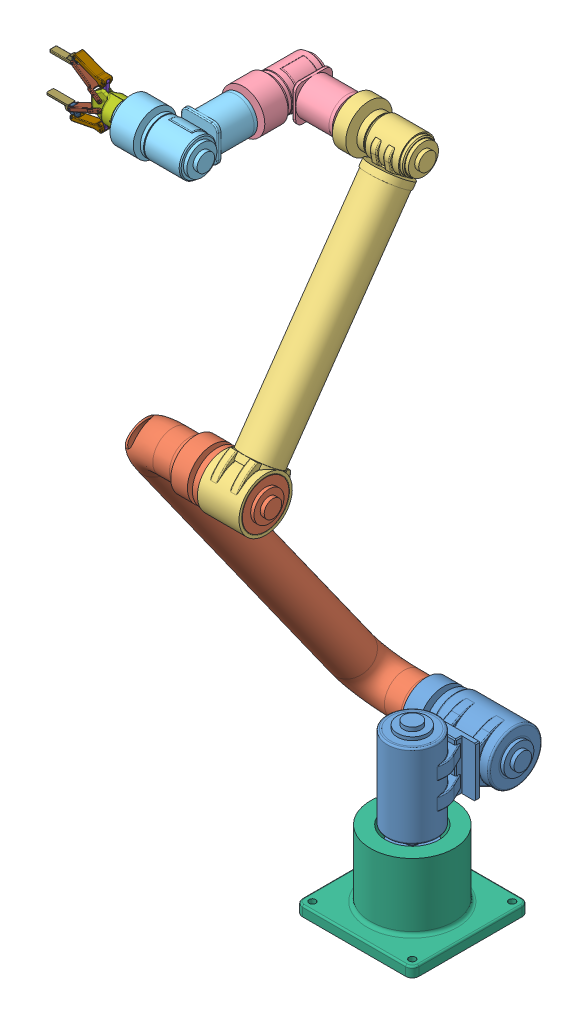
SolidWorks assembly qf_space_manipilator, configuration 默认. Lengths in mm.
Overall size (931.68 2266.25 1901.05).
18 component instances, 12 part files, 19 mates.
Components (placement in the parent):
- 1-1: 1 [默认] at (175 480 1283.54) x (1 0 0) z (0 -1 0) size (296.02 355 322)
- 2-1: 2 [默认] at (10.98 360 1083.54) x (0 -0.094498 0.995525) z (1 0 0) size (741.96 1181.19 535.98)
- 3-1: 3 [默认] at (167.5 1403.4778 1733.2672) x (0 0.572418 0.819962) z (0 0.819962 -0.572418) size (161.46 230.6 965)
- 4-1: 4 [默认] at (8.9 2006.1499 1312.54) x (0 1 0) z (1 0 0) size (130 235 470.6)
- 5-1: 5 [默认] at (763.6983 2411.2318 -1009.3375) x (-0.587026 0.762889 0.270927) z (-0.805463 -0.584033 -0.100675) size (262.23 449.62 237.88)
- Main_carrier_of_spool_cover_Varsay_X2_0131_X0_lan-1: Main_carrier_of_spool_cover_Varsay_X2_0131_X0_lan [默认] at (175 0 1283.54) x (0 0 1) z (0 1 0) size (350 350 230)
- Robotiq 2f-140-1: Robotiq 2f-140 [默认] at (-742.3808 2088.878 1773.5387) x (0.739353 0.591715 0.321296) z (0.557602 -0.805552 0.200415) size (250.11 134.48 238.85)
  - 2F-Body-1: 2F-Body [默认] at (218.7669 -271.2651 273.3125) x (0.593526 -0.031903 -0.804182) z (0.321296 0.925528 0.200415) size (89.6 94.04 75)
  - Finger1-1: Finger1 [默认] at (213.3406 -273.1738 290.8261) x (0.782068 -0.139996 -0.607265) z (0.321296 0.925528 0.200415) size (33.04 20.16 9.4)
  - Finger1-2: Finger1 [默认] at (225.7111 -272.8186 269.3539) x (-0.493154 -0.017144 0.869773) z (-0.321296 -0.925528 -0.200415) size (33.04 20.16 9.4)
  - Finger2-1: Finger2 [默认] at (213.3406 -273.1738 290.8261) x (0.782068 -0.139996 -0.607265) z (0.321296 0.925528 0.200415) size (58 91.26 27.21)
  - Finger4-1: Finger4 [默认] at (221.3264 -265.9336 244.5877) x (0.593526 -0.031903 -0.804182) z (0.321296 0.925528 0.200415) size (29.9 28.02 27)
  - Finger3-1: Finger3 [默认] at (208.6208 -271.1191 288.6542) x (0.782068 -0.139996 -0.607265) z (0.321296 0.925528 0.200415) size (78.86 86.37 35.78)
  - Fingertip-1: Fingertip [默认] at (221.3264 -265.9336 244.5877) x (0.593526 -0.031903 -0.804182) z (0.321296 0.925528 0.200415) size (19.16 65.5 22)
  - Finger2-2: Finger2 [默认] at (225.6469 -273.0037 269.3138) x (-0.493154 -0.017144 0.869773) z (-0.321296 -0.925528 -0.200415) size (58 91.26 27.21)
  - Finger4-2: Finger4 [默认] at (206.7467 -268.0999 276.9677) x (-0.593526 0.031903 0.804182) z (-0.321296 -0.925528 -0.200415) size (29.9 28.02 27)
  - Finger3-2: Finger3 [默认] at (166.9891 -256.8067 289.3008) x (0.856188 -0.374337 0.35611) z (0.321296 0.925528 0.200415) size (78.86 86.37 35.78)
  - Fingertip-2: Fingertip [默认] at (206.7467 -268.0999 276.9677) x (-0.593526 0.031903 0.804182) z (-0.321296 -0.925528 -0.200415) size (19.16 65.5 22)
Mates (geometry in assembly coordinates):
- 同心1: concentric anti-aligned: cylinder of 1-1 through (175 230 1283.54) axis (0 1 0) radius 75; cylinder of Main_carrier_of_spool_cover_Varsay_X2_0131_X0_lan-1 through (175 230 1283.54) axis (0 -1 0) radius 125
- 重合2: coincident anti-aligned: plane of 1-1 through (175 230 1283.54) normal (0 -1 0); plane of Main_carrier_of_spool_cover_Varsay_X2_0131_X0_lan-1 through (175 230 1283.54) normal (0 1 0)
- 同心3: concentric anti-aligned: cylinder of 1-1 through (115 360 1083.54) axis (1 0 0) radius 47.5; cylinder of 2-1 through (285 360 1083.54) axis (-1 0 0) radius 20
- 重合4: coincident anti-aligned: plane of 1-1 through (10.98 360 1083.54) normal (-1 0 0); plane of 2-1 through (10.98 360 1083.54) normal (1 0 0)
- 同心4: concentric anti-aligned: cylinder of 2-1 through (285 1337.8809 1779.0606) axis (-1 0 0) radius 70; cylinder of 3-1 through (105 1337.8809 1779.0606) axis (1 0 0) radius 70
- 重合5: coincident anti-aligned: plane of 2-1 through (105 1337.8809 1779.0606) normal (1 0 0); plane of 3-1 through (105 1337.8809 1779.0606) normal (-1 0 0)
- 同心6: concentric anti-aligned: cylinder of 3-1 through (18.9 2006.1499 1312.54) axis (1 0 0) radius 25; cylinder of 4-1 through (227.5 2006.1499 1312.54) axis (-1 0 0) radius 20
- 重合7: coincident anti-aligned: plane of 3-1 through (18.9 2006.1499 1312.54) normal (-1 0 0); plane of 4-1 through (18.9 2006.1499 1312.54) normal (1 0 0)
- 同心7: concentric anti-aligned: cylinder of 4-1 through (-158.1 2006.1499 1470.54) axis (0 0 -1) radius 20; cylinder of 5-1 through (-158.1 2006.1499 1261.94) axis (0 0 1) radius 20
- 重合8: coincident anti-aligned: plane of 4-1 through (-158.1 2006.1499 1470.54) normal (0 0 1); plane of 5-1 through (-158.1 2006.1499 1470.54) normal (0 0 -1)
- 平行1: parallel aligned: plane of 1-1 through (175 480 1183.54) normal (0 0 1); plane of Main_carrier_of_spool_cover_Varsay_X2_0131_X0_lan-1 through (350 30 1458.54) normal (0 0 1)
- 平行2: parallel aligned: plane of 1-1 through (285 360 1083.54) normal (1 0 0); plane of 2-1 through (230 1337.8809 1779.0606) normal (1 0 0)
- 平行3: parallel aligned: plane of 2-1 through (230 1337.8809 1779.0606) normal (1 0 0); plane of 3-1 through (237.5 2006.1499 1312.54) normal (1 0 0)
- 重合15: coincident anti-aligned: plane of Main_carrier_of_spool_cover_Varsay_X2_0131_X0_lan-1 through (0 30 1108.54) normal (-1 0 0)
- 重合16: coincident anti-aligned: plane of Main_carrier_of_spool_cover_Varsay_X2_0131_X0_lan-1 through (175 0 1283.54) normal (0 -1 0)
- 重合17: coincident anti-aligned: plane of 5-1 through (-326.0995 2006.5619 1647.54) normal (-0.999997 0.002452 0); plane of Robotiq 2f-140-1/2F-Body-1 through (-326.0971 2007.5275 1648.015) normal (0.999997 -0.002452 0)
- 同心9: concentric aligned: cylinder of 5-1 through (-326.0995 2006.5619 1647.54) axis (0.999997 -0.002452 0) radius 40; cylinder of Robotiq 2f-140-1/2F-Body-1 through (-397.8787 2006.7379 1647.54) axis (0.999997 -0.002452 0) radius 37.5
- 重合18: coincident aligned: plane of 4-1 through (-158.1 2006.1499 1458.54) normal (0 0 1); plane of Main_carrier_of_spool_cover_Varsay_X2_0131_X0_lan-1 through (350 30 1458.54) normal (0 0 1)
- 平行5: parallel aligned: plane of Main_carrier_of_spool_cover_Varsay_X2_0131_X0_lan-1 through (350 30 1458.54) normal (0 0 1); plane of Robotiq 2f-140-1/2F-Body-1 through (-387.2773 2006.7119 1658.54) normal (0 0 1)
